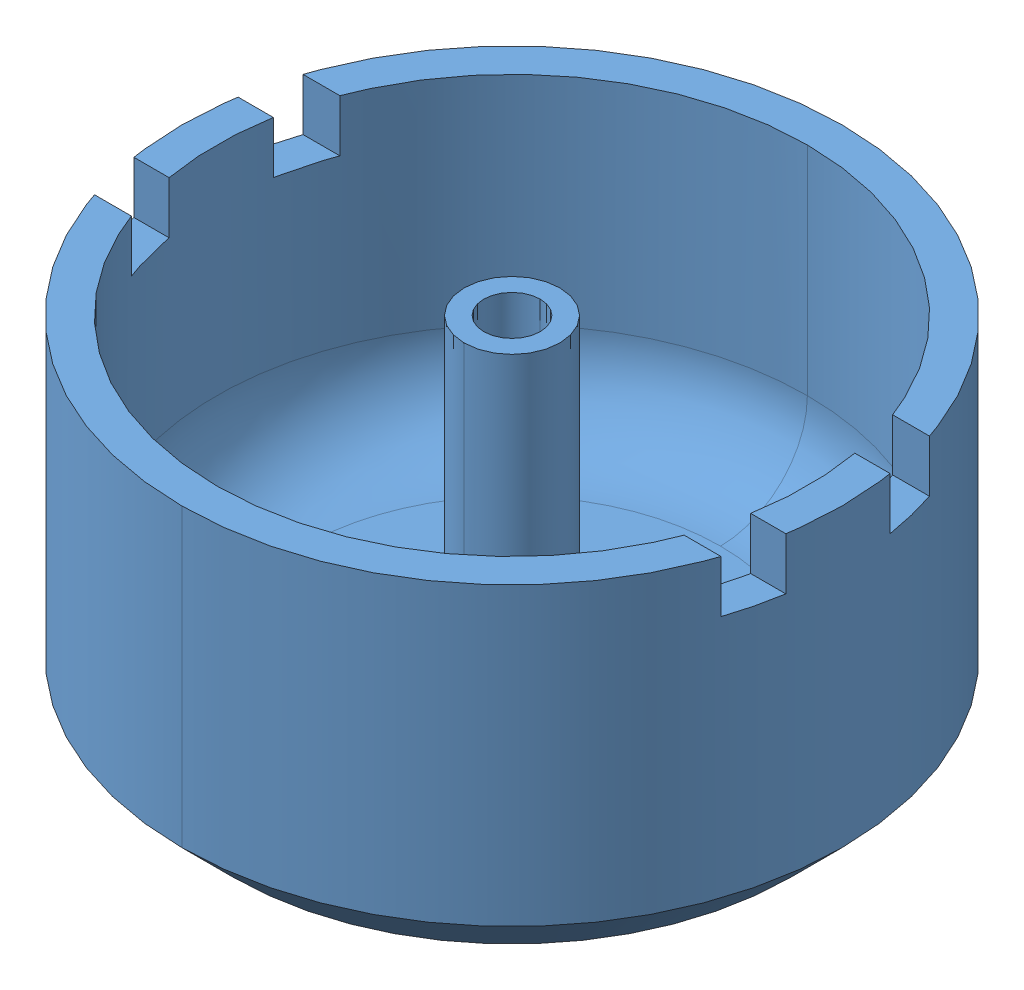
SolidWorks assembly Дроссель 38, configuration Default. Lengths in mm.
Overall size (38 20 38).
5 component instances, 3 part files, 0 mates.
Components (placement in the parent):
- Дроссель 38.STEP-1: Дроссель 38.STEP [Default] at origin size (47.39 28.45 38)
  - Корыто дросселя.STEP-1: Корыто дросселя.STEP [Default] at (662.6174 0 0) size (38 20 38)
  - Феррит 25х15х10,5.STEP-1: Феррит 25х15х10,5.STEP [Default] at (662.6174 0 0) size (32.62 16 32.28) (hidden)
  - Part1^Дроссель 38.STEP-1: Part1^Дроссель 38.STEP [Default] at (88.1826 -25.3339 337.2152) x (-0.46186 -0.012871 -0.886859) z (0.886159 0.035591 -0.462012) size (2.75 12.87 19.34) (hidden)
  - Part1^Дроссель 38.STEP-2: Part1^Дроссель 38.STEP [Default] at (61.1196 -26.088 -285.2489) x (0.46186 0.012871 -0.886859) z (0.886159 0.035591 0.462012) size (2.75 12.87 19.34) (hidden)
